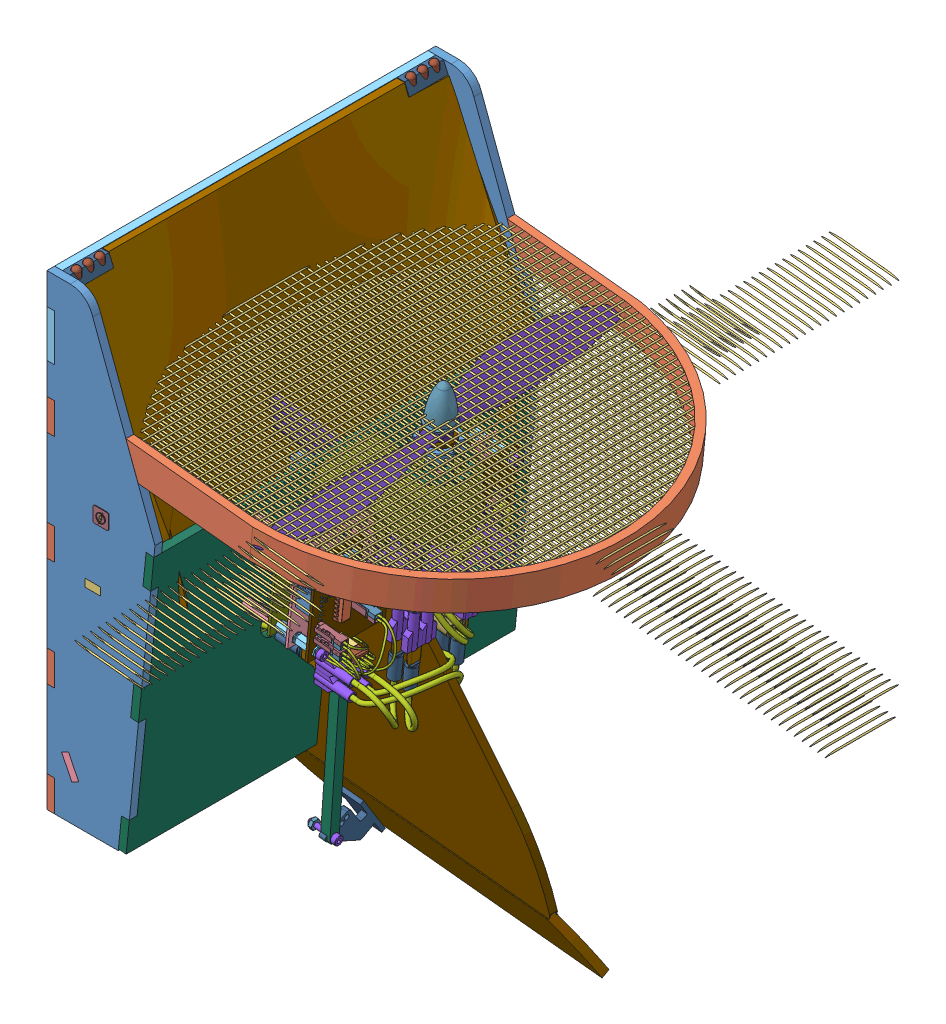
SolidWorks assembly AssTotaleSimu, configuration Défaut. Lengths in mm. (continued)
Components (placement in the parent): (continued)
- AssStructSimu-1: AssStructSimu [Défaut] at (-125.7658 -1.8483 624.6548) x (1 0 0) z (0 0 -1) size (323.53 326.04 251.6) (continued)
  - AssCarte-1: AssCarte [Défaut] at (-42.8534 32.2132 302.028) x (-0.101852 0.9948 0) z (0.9948 0.101852 0) size (91.19 130.57 98.45) (continued)
    - carte_onduleur_v4-1: carte_onduleur_v4 [Défaut] at (-25.7639 0.8332 112.9379) size (66.52 130.57 82.34) (continued)
      - C_DEC_COM1-1: C_DEC_COM1 [Défaut] at (-15 -36 0.803) x (0 -1 0) z (0 0 1) size (2.34 1.04 0.5) (continued)
        - Open CASCADE STEP translator 6.8 1.6.1-1: Open CASCADE STEP translator 6.8 1.6.1 [Défaut] at origin size (2.34 1.04 0.5)
          - Body_1-1: Body_1 [Défaut] at origin size (2.29 1.04 0.43)
          - Pin_1-1: Pin_1 [Défaut] at (0.3048 0 0) x (-1 0 0) z (0 0 1) size (0.51 1.02 0.5)
          - Pin_2-1: Pin_2 [Défaut] at origin size (0.51 1.02 0.5)
      - C_DEC_COMP2-1: C_DEC_COMP2 [Défaut] at (-13 -9.3 0.803) x (0 -1 0) z (0 0 1) size (2.34 1.04 0.5)
        - Open CASCADE STEP translator 6.8 1.6.1-1: Open CASCADE STEP translator 6.8 1.6.1 [Défaut] at origin size (2.34 1.04 0.5)
          - Body_1-1: Body_1 [Défaut] at origin size (2.29 1.04 0.43)
          - Pin_1-1: Pin_1 [Défaut] at (0.3048 0 0) x (-1 0 0) z (0 0 1) size (0.51 1.02 0.5)
          - Pin_2-1: Pin_2 [Défaut] at origin size (0.51 1.02 0.5)
      - C_DEC_COMP3-1: C_DEC_COMP3 [Défaut] at (-14.6 -22.9 0.803) x (0 -1 0) z (0 0 1) size (2.34 1.04 0.5)
        - Open CASCADE STEP translator 6.8 1.6.1-1: Open CASCADE STEP translator 6.8 1.6.1 [Défaut] at origin size (2.34 1.04 0.5)
          - Body_1-1: Body_1 [Défaut] at origin size (2.29 1.04 0.43)
          - Pin_1-1: Pin_1 [Défaut] at (0.3048 0 0) x (-1 0 0) z (0 0 1) size (0.51 1.02 0.5)
          - Pin_2-1: Pin_2 [Défaut] at origin size (0.51 1.02 0.5)
      - D_VBAT-1: D_VBAT [Défaut] at (-1.2 46.4 0.803) x (0 -1 0) z (0 0 1) size (2.34 1.04 0.5)
        - Open CASCADE STEP translator 6.8 1.6.1-1: Open CASCADE STEP translator 6.8 1.6.1 [Défaut] at origin size (2.34 1.04 0.5)
          - Body_1-1: Body_1 [Défaut] at origin size (2.29 1.04 0.43)
          - Pin_1-1: Pin_1 [Défaut] at (0.3048 0 0) x (-1 0 0) z (0 0 1) size (0.51 1.02 0.5)
          - Pin_2-1: Pin_2 [Défaut] at origin size (0.51 1.02 0.5)
      - D_3V-1: D_3V [Défaut] at (1.3 46.3 0.803) x (0 -1 0) z (0 0 1) size (2.34 1.04 0.5)
        - Open CASCADE STEP translator 6.8 1.6.1-1: Open CASCADE STEP translator 6.8 1.6.1 [Défaut] at origin size (2.34 1.04 0.5)
          - Body_1-1: Body_1 [Défaut] at origin size (2.29 1.04 0.43)
          - Pin_1-1: Pin_1 [Défaut] at (0.3048 0 0) x (-1 0 0) z (0 0 1) size (0.51 1.02 0.5)
          - Pin_2-1: Pin_2 [Défaut] at origin size (0.51 1.02 0.5)
      - D_5V-1: D_5V [Défaut] at (-3.7 46.4 0.803) x (0 -1 0) z (0 0 1) size (2.34 1.04 0.5)
        - Open CASCADE STEP translator 6.8 1.6.1-1: Open CASCADE STEP translator 6.8 1.6.1 [Défaut] at origin size (2.34 1.04 0.5)
          - Body_1-1: Body_1 [Défaut] at origin size (2.29 1.04 0.43)
          - Pin_1-1: Pin_1 [Défaut] at (0.3048 0 0) x (-1 0 0) z (0 0 1) size (0.51 1.02 0.5)
          - Pin_2-1: Pin_2 [Défaut] at origin size (0.51 1.02 0.5)
      - R1_1-1: R1_1 [Défaut] at (-20.2 -36.1 0.803) x (-1 0 0) z (0 0 1) size (2.34 1.04 0.5)
        - Open CASCADE STEP translator 6.8 1.12.1-1: Open CASCADE STEP translator 6.8 1.12.1 [Défaut] at origin size (2.34 1.04 0.5)
          - Body_1_3-1: Body_1_3 [Défaut] at origin size (2.29 1.04 0.43)
          - Pin_1_2-1: Pin_1_2 [Défaut] at (0.3048 0 0) x (-1 0 0) z (0 0 1) size (0.51 1.02 0.5)
          - Pin_2_2-1: Pin_2_2 [Défaut] at origin size (0.51 1.02 0.5)
      - R1_2-1: R1_2 [Défaut] at (-15.5 -34.6 0.803) x (-1 0 0) z (0 0 1) size (2.34 1.04 0.5)
        - Open CASCADE STEP translator 6.8 1.12.1-1: Open CASCADE STEP translator 6.8 1.12.1 [Défaut] at origin size (2.34 1.04 0.5)
          - Body_1_3-1: Body_1_3 [Défaut] at origin size (2.29 1.04 0.43)
          - Pin_1_2-1: Pin_1_2 [Défaut] at (0.3048 0 0) x (-1 0 0) z (0 0 1) size (0.51 1.02 0.5)
          - Pin_2_2-1: Pin_2_2 [Défaut] at origin size (0.51 1.02 0.5)
      - R1_3-1: R1_3 [Défaut] at (-20.3 -39.9 0.803) x (-1 0 0) z (0 0 1) size (2.34 1.04 0.5)
        - Open CASCADE STEP translator 6.8 1.12.1-1: Open CASCADE STEP translator 6.8 1.12.1 [Défaut] at origin size (2.34 1.04 0.5)
          - Body_1_3-1: Body_1_3 [Défaut] at origin size (2.29 1.04 0.43)
          - Pin_1_2-1: Pin_1_2 [Défaut] at (0.3048 0 0) x (-1 0 0) z (0 0 1) size (0.51 1.02 0.5)
          - Pin_2_2-1: Pin_2_2 [Défaut] at origin size (0.51 1.02 0.5)
      - R1_4-1: R1_4 [Défaut] at (-20.3 -38.1 0.803) x (-1 0 0) z (0 0 1) size (2.34 1.04 0.5)
        - Open CASCADE STEP translator 6.8 1.12.1-1: Open CASCADE STEP translator 6.8 1.12.1 [Défaut] at origin size (2.34 1.04 0.5)
          - Body_1_3-1: Body_1_3 [Défaut] at origin size (2.29 1.04 0.43)
          - Pin_1_2-1: Pin_1_2 [Défaut] at (0.3048 0 0) x (-1 0 0) z (0 0 1) size (0.51 1.02 0.5)
          - Pin_2_2-1: Pin_2_2 [Défaut] at origin size (0.51 1.02 0.5)
      - R1_5-1: R1_5 [Défaut] at (-17.1336 -39.7 0.803) size (2.34 1.04 0.5)
        - Open CASCADE STEP translator 6.8 1.12.1-1: Open CASCADE STEP translator 6.8 1.12.1 [Défaut] at origin size (2.34 1.04 0.5)
          - Body_1_3-1: Body_1_3 [Défaut] at origin size (2.29 1.04 0.43)
          - Pin_1_2-1: Pin_1_2 [Défaut] at (0.3048 0 0) x (-1 0 0) z (0 0 1) size (0.51 1.02 0.5)
          - Pin_2_2-1: Pin_2_2 [Défaut] at origin size (0.51 1.02 0.5)
      - R2_1-1: R2_1 [Défaut] at (-18.5 -9.5 0.803) x (-1 0 0) z (0 0 1) size (2.34 1.04 0.5)
        - Open CASCADE STEP translator 6.8 1.12.1-1: Open CASCADE STEP translator 6.8 1.12.1 [Défaut] at origin size (2.34 1.04 0.5)
          - Body_1_3-1: Body_1_3 [Défaut] at origin size (2.29 1.04 0.43)
          - Pin_1_2-1: Pin_1_2 [Défaut] at (0.3048 0 0) x (-1 0 0) z (0 0 1) size (0.51 1.02 0.5)
          - Pin_2_2-1: Pin_2_2 [Défaut] at origin size (0.51 1.02 0.5)
      - R2_2-1: R2_2 [Défaut] at (-13.1 -8 0.803) x (-1 0 0) z (0 0 1) size (2.34 1.04 0.5)
        - Open CASCADE STEP translator 6.8 1.12.1-1: Open CASCADE STEP translator 6.8 1.12.1 [Défaut] at origin size (2.34 1.04 0.5)
          - Body_1_3-1: Body_1_3 [Défaut] at origin size (2.29 1.04 0.43)
          - Pin_1_2-1: Pin_1_2 [Défaut] at (0.3048 0 0) x (-1 0 0) z (0 0 1) size (0.51 1.02 0.5)
          - Pin_2_2-1: Pin_2_2 [Défaut] at origin size (0.51 1.02 0.5)
      - R2_3-1: R2_3 [Défaut] at (-18.5 -11.2 0.803) x (-1 0 0) z (0 0 1) size (2.34 1.04 0.5)
        - Open CASCADE STEP translator 6.8 1.12.1-1: Open CASCADE STEP translator 6.8 1.12.1 [Défaut] at origin size (2.34 1.04 0.5)
          - Body_1_3-1: Body_1_3 [Défaut] at origin size (2.29 1.04 0.43)
          - Pin_1_2-1: Pin_1_2 [Défaut] at (0.3048 0 0) x (-1 0 0) z (0 0 1) size (0.51 1.02 0.5)
          - Pin_2_2-1: Pin_2_2 [Défaut] at origin size (0.51 1.02 0.5)
      - R2_4-1: R2_4 [Défaut] at (-18.5 -12.8 0.803) x (-1 0 0) z (0 0 1) size (2.34 1.04 0.5)
        - Open CASCADE STEP translator 6.8 1.12.1-1: Open CASCADE STEP translator 6.8 1.12.1 [Défaut] at origin size (2.34 1.04 0.5)
          - Body_1_3-1: Body_1_3 [Défaut] at origin size (2.29 1.04 0.43)
          - Pin_1_2-1: Pin_1_2 [Défaut] at (0.3048 0 0) x (-1 0 0) z (0 0 1) size (0.51 1.02 0.5)
          - Pin_2_2-1: Pin_2_2 [Défaut] at origin size (0.51 1.02 0.5)
      - R2_5-1: R2_5 [Défaut] at (-15.1336 -13 0.803) size (2.34 1.04 0.5)
        - Open CASCADE STEP translator 6.8 1.12.1-1: Open CASCADE STEP translator 6.8 1.12.1 [Défaut] at origin size (2.34 1.04 0.5)
          - Body_1_3-1: Body_1_3 [Défaut] at origin size (2.29 1.04 0.43)
          - Pin_1_2-1: Pin_1_2 [Défaut] at (0.3048 0 0) x (-1 0 0) z (0 0 1) size (0.51 1.02 0.5)
          - Pin_2_2-1: Pin_2_2 [Défaut] at origin size (0.51 1.02 0.5)
      - R3_1-1: R3_1 [Défaut] at (-19.9 -23.1 0.803) x (-1 0 0) z (0 0 1) size (2.34 1.04 0.5)
        - Open CASCADE STEP translator 6.8 1.12.1-1: Open CASCADE STEP translator 6.8 1.12.1 [Défaut] at origin size (2.34 1.04 0.5)
          - Body_1_3-1: Body_1_3 [Défaut] at origin size (2.29 1.04 0.43)
          - Pin_1_2-1: Pin_1_2 [Défaut] at (0.3048 0 0) x (-1 0 0) z (0 0 1) size (0.51 1.02 0.5)
          - Pin_2_2-1: Pin_2_2 [Défaut] at origin size (0.51 1.02 0.5)
      - R3_2-1: R3_2 [Défaut] at (-14.7 -21.6 0.803) x (-1 0 0) z (0 0 1) size (2.34 1.04 0.5)
        - Open CASCADE STEP translator 6.8 1.12.1-1: Open CASCADE STEP translator 6.8 1.12.1 [Défaut] at origin size (2.34 1.04 0.5)
          - Body_1_3-1: Body_1_3 [Défaut] at origin size (2.29 1.04 0.43)
          - Pin_1_2-1: Pin_1_2 [Défaut] at (0.3048 0 0) x (-1 0 0) z (0 0 1) size (0.51 1.02 0.5)
          - Pin_2_2-1: Pin_2_2 [Défaut] at origin size (0.51 1.02 0.5)
      - R3_3-1: R3_3 [Défaut] at (-19.9 -24.8 0.803) x (-1 0 0) z (0 0 1) size (2.34 1.04 0.5)
        - Open CASCADE STEP translator 6.8 1.12.1-1: Open CASCADE STEP translator 6.8 1.12.1 [Défaut] at origin size (2.34 1.04 0.5)
          - Body_1_3-1: Body_1_3 [Défaut] at origin size (2.29 1.04 0.43)
          - Pin_1_2-1: Pin_1_2 [Défaut] at (0.3048 0 0) x (-1 0 0) z (0 0 1) size (0.51 1.02 0.5)
          - Pin_2_2-1: Pin_2_2 [Défaut] at origin size (0.51 1.02 0.5)
      - R3_4-1: R3_4 [Défaut] at (-19.9 -26.4 0.803) x (-1 0 0) z (0 0 1) size (2.34 1.04 0.5)
        - Open CASCADE STEP translator 6.8 1.12.1-1: Open CASCADE STEP translator 6.8 1.12.1 [Défaut] at origin size (2.34 1.04 0.5)
          - Body_1_3-1: Body_1_3 [Défaut] at origin size (2.29 1.04 0.43)
          - Pin_1_2-1: Pin_1_2 [Défaut] at (0.3048 0 0) x (-1 0 0) z (0 0 1) size (0.51 1.02 0.5)
          - Pin_2_2-1: Pin_2_2 [Défaut] at origin size (0.51 1.02 0.5)
      - R3_5-1: R3_5 [Défaut] at (-16.7336 -26.5 0.803) size (2.34 1.04 0.5)
        - Open CASCADE STEP translator 6.8 1.12.1-1: Open CASCADE STEP translator 6.8 1.12.1 [Défaut] at origin size (2.34 1.04 0.5)
          - Body_1_3-1: Body_1_3 [Défaut] at origin size (2.29 1.04 0.43)
          - Pin_1_2-1: Pin_1_2 [Défaut] at (0.3048 0 0) x (-1 0 0) z (0 0 1) size (0.51 1.02 0.5)
          - Pin_2_2-1: Pin_2_2 [Défaut] at origin size (0.51 1.02 0.5)
      - R_LED_3V3-1: R_LED_3V3 [Défaut] at (1.3 47.9 0.803) x (0 1 0) z (0 0 1) size (2.34 1.04 0.5)
        - Open CASCADE STEP translator 6.8 1.12.1-1: Open CASCADE STEP translator 6.8 1.12.1 [Défaut] at origin size (2.34 1.04 0.5)
          - Body_1_3-1: Body_1_3 [Défaut] at origin size (2.29 1.04 0.43)
          - Pin_1_2-1: Pin_1_2 [Défaut] at (0.3048 0 0) x (-1 0 0) z (0 0 1) size (0.51 1.02 0.5)
          - Pin_2_2-1: Pin_2_2 [Défaut] at origin size (0.51 1.02 0.5)
      - R_LED_5V-1: R_LED_5V [Défaut] at (-3.7 47.7 0.803) x (0 1 0) z (0 0 1) size (2.34 1.04 0.5)
        - Open CASCADE STEP translator 6.8 1.12.1-1: Open CASCADE STEP translator 6.8 1.12.1 [Défaut] at origin size (2.34 1.04 0.5)
          - Body_1_3-1: Body_1_3 [Défaut] at origin size (2.29 1.04 0.43)
          - Pin_1_2-1: Pin_1_2 [Défaut] at (0.3048 0 0) x (-1 0 0) z (0 0 1) size (0.51 1.02 0.5)
          - Pin_2_2-1: Pin_2_2 [Défaut] at origin size (0.51 1.02 0.5)
      - R_LED_VBAT-1: R_LED_VBAT [Défaut] at (-1.2 47.9 0.803) x (0 1 0) z (0 0 1) size (2.34 1.04 0.5)
        - Open CASCADE STEP translator 6.8 1.12.1-1: Open CASCADE STEP translator 6.8 1.12.1 [Défaut] at origin size (2.34 1.04 0.5)
          - Body_1_3-1: Body_1_3 [Défaut] at origin size (2.29 1.04 0.43)
          - Pin_1_2-1: Pin_1_2 [Défaut] at (0.3048 0 0) x (-1 0 0) z (0 0 1) size (0.51 1.02 0.5)
          - Pin_2_2-1: Pin_2_2 [Défaut] at origin size (0.51 1.02 0.5)
      - CARTE_ALIM-1: CARTE_ALIM [Défaut] at (-6.4 -57.2 0.803) size (60 130 18.35)
        - Open CASCADE STEP translator 6.8 1.63.1-1: Open CASCADE STEP translator 6.8 1.63.1 [Défaut] at origin size (60 130 18.35)
          - Body_1_6-1: Body_1_6 [Défaut] at (7 56 -12) size (60 130 18.35)
            - 1_3-1: 1_3 [Défaut] at origin size (60 130 1.61)
            - 13_3-1: 13_3 [Défaut] at (0.4717 -40.93 0.803) x (0 1 0) z (0 0 1) size (5.65 4.9 1.7)
              - =_[0_1_1_4]_3-1: =_[0_1_1_4]_3 [Défaut] at origin size (5.65 4.9 1.7)
                - 2-1: 2 [Défaut] at origin size (3.75 4.9 1.53)
                - 3-1: 3 [Défaut] at origin size (0.95 0.51 1.06)
                - 4-1: 4 [Défaut] at origin size (0.95 0.51 1.06)
                - 5_2-1: 5_2 [Défaut] at origin size (0.95 0.51 1.06)
                - 6-1: 6 [Défaut] at origin size (0.95 0.51 1.06)
                - 7-1: 7 [Défaut] at (10.8 -5.08 0) x (-1 0 0) z (0 0 1) size (0.95 0.51 1.06)
                - 8_2-1: 8_2 [Défaut] at (10.8 -2.54 0) x (-1 0 0) z (0 0 1) size (0.95 0.51 1.06)
                - 9-1: 9 [Défaut] at (10.8 0 0) x (-1 0 0) z (0 0 1) size (0.95 0.51 1.06)
                - 10-1: 10 [Défaut] at (10.8 2.54 0) x (-1 0 0) z (0 0 1) size (0.95 0.51 1.06)
                - 11_2-1: 11_2 [Défaut] at (5.4 -1.27 0) x (-1 0 0) z (0 0 1) size (4.25 2.34 1.06)
            - 18-1: 18 [Défaut] at (-2.5283 -37.23 0.803) x (0 -1 0) z (0 0 1) size (2.34 1.04 0.5)
              - =_[0_1_1_16]-1: =_[0_1_1_16] [Défaut] at origin size (2.34 1.04 0.5)
                - 14_2-1: 14_2 [Défaut] at origin size (2.29 1.04 0.43)
                - 15_2-1: 15_2 [Défaut] at (0.3048 0 0) x (-1 0 0) z (0 0 1) size (0.51 1.02 0.5)
                - 16_2-1: 16_2 [Défaut] at origin size (0.51 1.02 0.5)
            - 21_2-1: 21_2 [Défaut] at (-2.2263 -24.628 -0.803) x (1 0 0) z (0 0 -1) size (8.01 8 14.24)
              - =_[0_1_1_21]-1: =_[0_1_1_21] [Défaut] at origin size (8.01 8 14.24)
                - 19-1: 19 [Défaut] at (1.8 0 0) x (1 0 0) z (0 -1 0) size (8.01 14.24 8)
            - 23_2-1: 23_2 [Défaut] at (1.2381 -31.53 0.803) size (2.34 1.04 0.5)
              - =_[0_1_1_16]-1: =_[0_1_1_16] [Défaut] at origin size (2.34 1.04 0.5)
                - 14_2-1: 14_2 [Défaut] at origin size (2.29 1.04 0.43)
                - 15_2-1: 15_2 [Défaut] at (0.3048 0 0) x (-1 0 0) z (0 0 1) size (0.51 1.02 0.5)
                - 16_2-1: 16_2 [Défaut] at origin size (0.51 1.02 0.5)
            - 28-1: 28 [Défaut] at (5 29.8636 0.803) x (0 -1 0) z (0 0 1) size (3.35 1.3 0.55)
              - =_[0_1_1_25]_2-1: =_[0_1_1_25]_2 [Défaut] at origin size (3.35 1.3 0.55)
                - 24-1: 24 [Défaut] at origin size (3.3 1.3 0.48)
                - 25_2-1: 25_2 [Défaut] at (0.5588 0 0) x (-1 0 0) z (0 0 1) size (0.76 1.27 0.55)
                - 26_2-1: 26_2 [Défaut] at origin size (0.76 1.27 0.55)
            - 30-1: 30 [Défaut] at (6.7 29.8636 0.803) x (0 -1 0) z (0 0 1) size (2.34 1.04 0.5)
              - =_[0_1_1_16]-1: =_[0_1_1_16] [Défaut] at origin size (2.34 1.04 0.5)
                - 14_2-1: 14_2 [Défaut] at origin size (2.29 1.04 0.43)
                - 15_2-1: 15_2 [Défaut] at (0.3048 0 0) x (-1 0 0) z (0 0 1) size (0.51 1.02 0.5)
                - 16_2-1: 16_2 [Défaut] at origin size (0.51 1.02 0.5)
            - 35_2-1: 35_2 [Défaut] at (-2.5 -46.37 0.803) x (0 1 0) z (0 0 1) size (3.4 2.06 0.79)
              - =_[0_1_1_31]-1: =_[0_1_1_31] [Défaut] at origin size (3.4 2.06 0.79)
                - 31_2-1: 31_2 [Défaut] at origin size (3.3 2.06 0.69)
                - 32_3-1: 32_3 [Défaut] at (0.5588 0 0) x (-1 0 0) z (0 0 1) size (0.81 2.03 0.79)
                - 33_3-1: 33_3 [Défaut] at origin size (0.81 2.03 0.79)
            - 37-1: 37 [Défaut] at (5 31.43 0.803) x (0 1 0) z (0 0 1) size (2.34 1.04 0.5)
              - =_[0_1_1_16]-1: =_[0_1_1_16] [Défaut] at origin size (2.34 1.04 0.5)
                - 14_2-1: 14_2 [Défaut] at origin size (2.29 1.04 0.43)
                - 15_2-1: 15_2 [Défaut] at (0.3048 0 0) x (-1 0 0) z (0 0 1) size (0.51 1.02 0.5)
                - 16_2-1: 16_2 [Défaut] at origin size (0.51 1.02 0.5)
            - 39-1: 39 [Défaut] at (-0.2 35.63 0.803) x (-1 0 0) z (0 0 1) size (2.34 1.04 0.5)
              - =_[0_1_1_16]-1: =_[0_1_1_16] [Défaut] at origin size (2.34 1.04 0.5)
                - 14_2-1: 14_2 [Défaut] at origin size (2.29 1.04 0.43)
                - 15_2-1: 15_2 [Défaut] at (0.3048 0 0) x (-1 0 0) z (0 0 1) size (0.51 1.02 0.5)
                - 16_2-1: 16_2 [Défaut] at origin size (0.51 1.02 0.5)
            - 41-1: 41 [Défaut] at (2.9 -45.5036 0.803) x (0 1 0) z (0 0 1) size (2.34 1.04 0.5)
              - =_[0_1_1_16]-1: =_[0_1_1_16] [Défaut] at origin size (2.34 1.04 0.5)
                - 14_2-1: 14_2 [Défaut] at origin size (2.29 1.04 0.43)
                - 15_2-1: 15_2 [Défaut] at (0.3048 0 0) x (-1 0 0) z (0 0 1) size (0.51 1.02 0.5)
                - 16_2-1: 16_2 [Défaut] at origin size (0.51 1.02 0.5)
            - 43-1: 43 [Défaut] at (17.1348 -42.6272 0.803) x (0 1 0) z (0 0 1) size (2.34 1.04 0.5)
              - =_[0_1_1_16]-1: =_[0_1_1_16] [Défaut] at origin size (2.34 1.04 0.5)
                - 14_2-1: 14_2 [Défaut] at origin size (2.29 1.04 0.43)
                - 15_2-1: 15_2 [Défaut] at (0.3048 0 0) x (-1 0 0) z (0 0 1) size (0.51 1.02 0.5)
                - 16_2-1: 16_2 [Défaut] at origin size (0.51 1.02 0.5)
            - 48_2-1: 48_2 [Défaut] at (-5.4717 -39.01 0.803) x (-1 0 0) z (0 0 1) size (4.19 3.4 1.75)
              - =_[0_1_1_40]-1: =_[0_1_1_40] [Défaut] at origin size (4.19 3.4 1.75)
                - 44_2-1: 44_2 [Défaut] at origin size (3.75 3.38 1.73)
                - 45_2-1: 45_2 [Défaut] at (0.438 0 0) x (-1 0 0) z (0 0 1) size (0.53 3.4 1.75)
                - 46-1: 46 [Défaut] at origin size (0.52 3.4 1.75)
            - 53-1: 53 [Défaut] at (0.9 35.63 0.803) size (2.34 1.04 0.5)
              - =_[0_1_1_45]-1: =_[0_1_1_45] [Défaut] at origin size (2.34 1.04 0.5)
                - 49_3-1: 49_3 [Défaut] at origin size (2.29 1.04 0.43)
                - 50-1: 50 [Défaut] at (0.3048 0 0) x (-1 0 0) z (0 0 1) size (0.51 1.02 0.5)
                - 51-1: 51 [Défaut] at origin size (0.51 1.02 0.5)
            - 55_2-1: 55_2 [Défaut] at (1.3 -45.5036 0.803) x (0 1 0) z (0 0 1) size (2.34 1.04 0.5)
              - =_[0_1_1_45]-1: =_[0_1_1_45] [Défaut] at origin size (2.34 1.04 0.5)
                - 49_3-1: 49_3 [Défaut] at origin size (2.29 1.04 0.43)
                - 50-1: 50 [Défaut] at (0.3048 0 0) x (-1 0 0) z (0 0 1) size (0.51 1.02 0.5)
                - 51-1: 51 [Défaut] at origin size (0.51 1.02 0.5)
            - 57_3-1: 57_3 [Défaut] at (17.2348 -43.9936 0.803) x (0 -1 0) z (0 0 1) size (2.34 1.04 0.5)
              - =_[0_1_1_45]-1: =_[0_1_1_45] [Défaut] at origin size (2.34 1.04 0.5)
                - 49_3-1: 49_3 [Défaut] at origin size (2.29 1.04 0.43)
                - 50-1: 50 [Défaut] at (0.3048 0 0) x (-1 0 0) z (0 0 1) size (0.51 1.02 0.5)
                - 51-1: 51 [Défaut] at origin size (0.51 1.02 0.5)
            - 65-1: 65 [Défaut] at (-4.8 30.93 0.803) x (-1 0 0) z (0 0 1) size (14.64 9.83 4.25)
              - =_[0_1_1_52]-1: =_[0_1_1_52] [Défaut] at origin size (14.64 9.83 4.25)
                - 63_2-1: 63_2 [Défaut] at (3 0 0) x (0 -1 0) z (0 0 1) size (9.83 14.64 4.25)
                  - =_[0_1_1_3]_5-1: =_[0_1_1_3]_5 [Défaut] at origin size (9.83 9.05 4.21)
                  - =_[0_1_1_4]_5-1: =_[0_1_1_4]_5 [Défaut] at origin size (9.48 7.76 1.21)
                  - =_[0_1_1_5]_5-1: =_[0_1_1_5]_5 [Défaut] at origin size (1.36 6.01 3.08)
                  - =_[0_1_1_6]_3-1: =_[0_1_1_6]_3 [Défaut] at origin size (1.36 6.01 3.08)
                  - =_[0_1_1_7]_3-1: =_[0_1_1_7]_3 [Défaut] at origin size (1.06 6.01 3.08)
            - 67-1: 67 [Défaut] at (13.5933 -37.5272 0.803) x (-1 0 0) z (0 0 1) size (2.34 1.04 0.5)
              - =_[0_1_1_16]-1: =_[0_1_1_16] [Défaut] at origin size (2.34 1.04 0.5)
                - 14_2-1: 14_2 [Défaut] at origin size (2.29 1.04 0.43)
                - 15_2-1: 15_2 [Défaut] at (0.3048 0 0) x (-1 0 0) z (0 0 1) size (0.51 1.02 0.5)
                - 16_2-1: 16_2 [Défaut] at origin size (0.51 1.02 0.5)
            - 70_2-1: 70_2 [Défaut] at (18.2733 -29.7272 0.803) x (0 1 0) z (0 0 1) size (6.06 4.95 1.88)
              - =_[0_1_1_61]-1: =_[0_1_1_61] [Défaut] at origin size (6.06 4.95 1.88)
                - 68-1: 68 [Défaut] x (1 0 0) z (0 -1 0) size (6.06 1.88 4.95)
            - 83-1: 83 [Défaut] at (-21.2 -38.07 0.803) x (-1 0 0) z (0 0 1) size (2.7 5.2 1.11)
              - =_[0_1_1_64]-1: =_[0_1_1_64] [Défaut] at origin size (2.7 5.2 1.11)
                - 84_2-1: 84_2 [Défaut] at (1.2 -4 0) x (0 1 0) z (0 0 1) size (5.2 2.7 1.11)
                  - =_[0_1_1_3]_6-1: =_[0_1_1_3]_6 [Défaut] at origin size (0.39 0.64 0.01)
                  - =_[0_1_1_4]_6-1: =_[0_1_1_4]_6 [Défaut] at origin size (0.6 1.9 0.2)
                  - =_[0_1_1_5]_6-1: =_[0_1_1_5]_6 [Défaut] at origin size (0.21 0.08 0.01)
                  - =_[0_1_1_6]_4-1: =_[0_1_1_6]_4 [Défaut] at origin size (0.6 1.9 0.2)
                  - =_[0_1_1_7]_4-1: =_[0_1_1_7]_4 [Défaut] at origin size (0.46 0.68 0.01)
                  - =_[0_1_1_8]_3-1: =_[0_1_1_8]_3 [Défaut] at origin size (0.38 0.66 0.01)
                  - =_[0_1_1_9]_2-1: =_[0_1_1_9]_2 [Défaut] at origin size (0.2 0.62 0.01)
                  - =_[0_1_1_10]_2-1: =_[0_1_1_10]_2 [Défaut] at origin size (4 2.7 1.1)
                  - =_[0_1_1_11]_2-1: =_[0_1_1_11]_2 [Défaut] at origin size (0.46 0.63 0.01)
                  - =_[0_1_1_12]_2-1: =_[0_1_1_12]_2 [Défaut] at origin size (0.56 0.68 0.01)
            - 86_2-1: 86_2 [Défaut] at (12.8933 -35.4272 0.803) x (0 1 0) z (0 0 1) size (2.7 5.2 1.11)
              - =_[0_1_1_77]-1: =_[0_1_1_77] [Défaut] at origin size (2.7 5.2 1.11)
                - 84_2-1: 84_2 [Défaut] at (1.2 -4 0) x (0 1 0) z (0 0 1) size (5.2 2.7 1.11)
                  - =_[0_1_1_3]_6-1: =_[0_1_1_3]_6 [Défaut] at origin size (0.39 0.64 0.01)
                  - =_[0_1_1_4]_6-1: =_[0_1_1_4]_6 [Défaut] at origin size (0.6 1.9 0.2)
                  - =_[0_1_1_5]_6-1: =_[0_1_1_5]_6 [Défaut] at origin size (0.21 0.08 0.01)
                  - =_[0_1_1_6]_4-1: =_[0_1_1_6]_4 [Défaut] at origin size (0.6 1.9 0.2)
                  - =_[0_1_1_7]_4-1: =_[0_1_1_7]_4 [Défaut] at origin size (0.46 0.68 0.01)
                  - =_[0_1_1_8]_3-1: =_[0_1_1_8]_3 [Défaut] at origin size (0.38 0.66 0.01)
                  - =_[0_1_1_9]_2-1: =_[0_1_1_9]_2 [Défaut] at origin size (0.2 0.62 0.01)
                  - =_[0_1_1_10]_2-1: =_[0_1_1_10]_2 [Défaut] at origin size (4 2.7 1.1)
                  - =_[0_1_1_11]_2-1: =_[0_1_1_11]_2 [Défaut] at origin size (0.46 0.63 0.01)
                  - =_[0_1_1_12]_2-1: =_[0_1_1_12]_2 [Défaut] at origin size (0.56 0.68 0.01)
            - 92_2-1: 92_2 [Défaut] at (20.9933 -39.3272 0.803) x (0 -1 0) z (0 0 1) size (2.79 1.98 0.64)
              - =_[0_1_1_79]-1: =_[0_1_1_79] [Défaut] at origin size (2.79 1.98 0.64)
                - 87-1: 87 [Défaut] at origin size (2.79 1.02 0.58)
                - 88-1: 88 [Défaut] x (0 -1 0) z (0 0 1) size (0.42 0.38 0.38)
                - 89-1: 89 [Défaut] at (-2.8448 -0.9652 0) x (0 1 0) z (0 0 1) size (0.55 0.38 0.38)
                - 90-1: 90 [Défaut] at (-0.9652 -2.8448 0) x (0 1 0) z (0 0 1) size (0.55 0.38 0.38)
            - 98-1: 98 [Défaut] at (-17.7 -48.47 0.803) x (0 -1 0) z (0 0 1) size (2.54 1.98 0.64)
              - =_[0_1_1_85]-1: =_[0_1_1_85] [Défaut] at origin size (2.54 1.98 0.64)
                - 93-1: 93 [Défaut] at origin size (2.54 1.14 0.58)
                - 94-1: 94 [Défaut] x (0 -1 0) z (0 0 1) size (0.43 0.51 0.38)
                - 95-1: 95 [Défaut] at (1.8796 1.8796 0) x (0 -1 0) z (0 0 1) size (0.43 0.51 0.38)
                - 96-1: 96 [Défaut] at (-0.9652 -2.8448 0) x (0 1 0) z (0 0 1) size (0.41 0.51 0.38)
            - 100-1: 100 [Défaut] at (24.3933 -43.2272 0.803) size (2.79 1.98 0.64)
              - =_[0_1_1_79]-1: =_[0_1_1_79] [Défaut] at origin size (2.79 1.98 0.64)
                - 87-1: 87 [Défaut] at origin size (2.79 1.02 0.58)
                - 88-1: 88 [Défaut] x (0 -1 0) z (0 0 1) size (0.42 0.38 0.38)
                - 89-1: 89 [Défaut] at (-2.8448 -0.9652 0) x (0 1 0) z (0 0 1) size (0.55 0.38 0.38)
                - 90-1: 90 [Défaut] at (-0.9652 -2.8448 0) x (0 1 0) z (0 0 1) size (0.55 0.38 0.38)
            - 102-1: 102 [Défaut] at (21.4933 -44.4272 0.803) x (0 -1 0) z (0 0 1) size (2.79 1.98 0.64)
              - =_[0_1_1_79]-1: =_[0_1_1_79] [Défaut] at origin size (2.79 1.98 0.64)
                - 87-1: 87 [Défaut] at origin size (2.79 1.02 0.58)
                - 88-1: 88 [Défaut] x (0 -1 0) z (0 0 1) size (0.42 0.38 0.38)
                - 89-1: 89 [Défaut] at (-2.8448 -0.9652 0) x (0 1 0) z (0 0 1) size (0.55 0.38 0.38)
                - 90-1: 90 [Défaut] at (-0.9652 -2.8448 0) x (0 1 0) z (0 0 1) size (0.55 0.38 0.38)
            - 107-1: 107 [Défaut] at (23.1933 -29.1272 -0.803) x (0 1 0) z (0 0 -1) size (9.6 14.35 5)
              - =_[0_1_1_93]-1: =_[0_1_1_93] [Défaut] at origin size (9.6 14.35 5)
                - 105-1: 105 [Défaut] at (0.5 -1 2) x (-1 0 0) z (0 0 1) size (9.6 14.35 5)
                  - =_[0_1_1_3]_7-1: =_[0_1_1_3]_7 [Défaut] at origin size (9.6 12.75 5)
                  - =_[0_1_1_4]_7-1: =_[0_1_1_4]_7 [Défaut] at origin size (2.2 1.6 2.2)
            - 109-1: 109 [Défaut] at (25.4933 -41.1272 0.803) x (-1 0 0) z (0 0 1) size (2.34 1.04 0.5)
              - =_[0_1_1_45]-1: =_[0_1_1_45] [Défaut] at origin size (2.34 1.04 0.5)
                - 49_3-1: 49_3 [Défaut] at origin size (2.29 1.04 0.43)
                - 50-1: 50 [Défaut] at (0.3048 0 0) x (-1 0 0) z (0 0 1) size (0.51 1.02 0.5)
                - 51-1: 51 [Défaut] at origin size (0.51 1.02 0.5)
            - 111-1: 111 [Défaut] at (22.0269 -41.8272 0.803) x (-1 0 0) z (0 0 1) size (2.34 1.04 0.5)
              - =_[0_1_1_45]-1: =_[0_1_1_45] [Défaut] at origin size (2.34 1.04 0.5)
                - 49_3-1: 49_3 [Défaut] at origin size (2.29 1.04 0.43)
                - 50-1: 50 [Défaut] at (0.3048 0 0) x (-1 0 0) z (0 0 1) size (0.51 1.02 0.5)
                - 51-1: 51 [Défaut] at origin size (0.51 1.02 0.5)
            - 113-1: 113 [Défaut] at (-24.8 -36.7036 0.803) x (0 1 0) z (0 0 1) size (2.34 1.04 0.5)
              - =_[0_1_1_45]-1: =_[0_1_1_45] [Défaut] at origin size (2.34 1.04 0.5)
                - 49_3-1: 49_3 [Défaut] at origin size (2.29 1.04 0.43)
                - 50-1: 50 [Défaut] at (0.3048 0 0) x (-1 0 0) z (0 0 1) size (0.51 1.02 0.5)
                - 51-1: 51 [Défaut] at origin size (0.51 1.02 0.5)
            - 115-1: 115 [Défaut] at (-24.8 -40.3036 0.803) x (0 1 0) z (0 0 1) size (2.34 1.04 0.5)
              - =_[0_1_1_45]-1: =_[0_1_1_45] [Défaut] at origin size (2.34 1.04 0.5)
                - 49_3-1: 49_3 [Défaut] at origin size (2.29 1.04 0.43)
                - 50-1: 50 [Défaut] at (0.3048 0 0) x (-1 0 0) z (0 0 1) size (0.51 1.02 0.5)
                - 51-1: 51 [Défaut] at origin size (0.51 1.02 0.5)
            - 117-1: 117 [Défaut] at (-16 -48.27 0.803) x (0 -1 0) z (0 0 1) size (2.34 1.04 0.5)
              - =_[0_1_1_45]-1: =_[0_1_1_45] [Défaut] at origin size (2.34 1.04 0.5)
                - 49_3-1: 49_3 [Défaut] at origin size (2.29 1.04 0.43)
                - 50-1: 50 [Défaut] at (0.3048 0 0) x (-1 0 0) z (0 0 1) size (0.51 1.02 0.5)
                - 51-1: 51 [Défaut] at origin size (0.51 1.02 0.5)
            - 119-1: 119 [Défaut] at (-22.5189 -47.87 0.803) x (-1 0 0) z (0 0 1) size (2.34 1.04 0.5)
              - =_[0_1_1_45]-1: =_[0_1_1_45] [Défaut] at origin size (2.34 1.04 0.5)
                - 49_3-1: 49_3 [Défaut] at origin size (2.29 1.04 0.43)
                - 50-1: 50 [Défaut] at (0.3048 0 0) x (-1 0 0) z (0 0 1) size (0.51 1.02 0.5)
                - 51-1: 51 [Défaut] at origin size (0.51 1.02 0.5)
            - 121-1: 121 [Défaut] at (22.3933 -38.9272 0.803) size (2.34 1.04 0.5)
              - =_[0_1_1_45]-1: =_[0_1_1_45] [Défaut] at origin size (2.34 1.04 0.5)
                - 49_3-1: 49_3 [Défaut] at origin size (2.29 1.04 0.43)
                - 50-1: 50 [Défaut] at (0.3048 0 0) x (-1 0 0) z (0 0 1) size (0.51 1.02 0.5)
                - 51-1: 51 [Défaut] at origin size (0.51 1.02 0.5)
            - 123-1: 123 [Défaut] at (22.0933 -36.4272 0.803) x (-1 0 0) z (0 0 1) size (2.34 1.04 0.5)
              - =_[0_1_1_45]-1: =_[0_1_1_45] [Défaut] at origin size (2.34 1.04 0.5)
                - 49_3-1: 49_3 [Défaut] at origin size (2.29 1.04 0.43)
                - 50-1: 50 [Défaut] at (0.3048 0 0) x (-1 0 0) z (0 0 1) size (0.51 1.02 0.5)
                - 51-1: 51 [Défaut] at origin size (0.51 1.02 0.5)
            - 125-1: 125 [Défaut] at (22.3933 -32.0272 0.803) x (0 -1 0) z (0 0 1) size (2.34 1.04 0.5)
              - =_[0_1_1_45]-1: =_[0_1_1_45] [Défaut] at origin size (2.34 1.04 0.5)
                - 49_3-1: 49_3 [Défaut] at origin size (2.29 1.04 0.43)
                - 50-1: 50 [Défaut] at (0.3048 0 0) x (-1 0 0) z (0 0 1) size (0.51 1.02 0.5)
                - 51-1: 51 [Défaut] at origin size (0.51 1.02 0.5)
            - 127-1: 127 [Défaut] at (17.9597 -23.1272 0.803) size (2.34 1.04 0.5)
              - =_[0_1_1_16]-1: =_[0_1_1_16] [Défaut] at origin size (2.34 1.04 0.5)
                - 14_2-1: 14_2 [Défaut] at origin size (2.29 1.04 0.43)
                - 15_2-1: 15_2 [Défaut] at (0.3048 0 0) x (-1 0 0) z (0 0 1) size (0.51 1.02 0.5)
                - 16_2-1: 16_2 [Défaut] at origin size (0.51 1.02 0.5)
            - 129-1: 129 [Défaut] at (20.0269 -24.9272 0.803) x (-1 0 0) z (0 0 1) size (2.34 1.04 0.5)
              - =_[0_1_1_16]-1: =_[0_1_1_16] [Défaut] at origin size (2.34 1.04 0.5)
                - 14_2-1: 14_2 [Défaut] at origin size (2.29 1.04 0.43)
                - 15_2-1: 15_2 [Défaut] at (0.3048 0 0) x (-1 0 0) z (0 0 1) size (0.51 1.02 0.5)
                - 16_2-1: 16_2 [Défaut] at origin size (0.51 1.02 0.5)
            - 131-1: 131 [Défaut] at (16.9933 -37.5272 0.803) x (-1 0 0) z (0 0 1) size (2.34 1.04 0.5)
              - =_[0_1_1_45]-1: =_[0_1_1_45] [Défaut] at origin size (2.34 1.04 0.5)
                - 49_3-1: 49_3 [Défaut] at origin size (2.29 1.04 0.43)
                - 50-1: 50 [Défaut] at (0.3048 0 0) x (-1 0 0) z (0 0 1) size (0.51 1.02 0.5)
                - 51-1: 51 [Défaut] at origin size (0.51 1.02 0.5)
            - 136-1: 136 [Défaut] at (3.2957 -29.23 0.803) x (-1 0 0) z (0 0 1) size (4.78 2.79 2.03)
              - =_[0_1_1_110]_2-1: =_[0_1_1_110]_2 [Défaut] at origin size (4.78 2.79 2.03)
                - 132-1: 132 [Défaut] at origin size (4.32 2.79 1.78)
                - 133-1: 133 [Défaut] at (0.4572 0 0) x (-1 0 0) z (0 0 1) size (1.02 1.27 1.32)
                - 134-1: 134 [Défaut] at origin size (1.02 1.27 1.32)
            - 141-1: 141 [Défaut] at (0.2436 -33.3673 0.803) size (3.35 1.3 0.55)
              - =_[0_1_1_115]_2-1: =_[0_1_1_115]_2 [Défaut] at origin size (3.35 1.3 0.55)
                - 137-1: 137 [Défaut] at origin size (3.3 1.3 0.48)
                - 138-1: 138 [Défaut] at (0.5588 0 0) x (-1 0 0) z (0 0 1) size (0.76 1.27 0.55)
                - 139-1: 139 [Défaut] at origin size (0.76 1.27 0.55)
            - 143_2-1: 143_2 [Défaut] at (-0.3 -45.47 0.803) x (0 1 0) z (0 0 1) size (2.34 1.04 0.5)
              - =_[0_1_1_16]-1: =_[0_1_1_16] [Défaut] at origin size (2.34 1.04 0.5)
                - 14_2-1: 14_2 [Défaut] at origin size (2.29 1.04 0.43)
                - 15_2-1: 15_2 [Défaut] at (0.3048 0 0) x (-1 0 0) z (0 0 1) size (0.51 1.02 0.5)
                - 16_2-1: 16_2 [Défaut] at origin size (0.51 1.02 0.5)
            - 145-1: 145 [Défaut] at (6.6 31.13 0.803) x (0 1 0) z (0 0 1) size (3.35 1.3 0.55)
              - =_[0_1_1_25]_2-1: =_[0_1_1_25]_2 [Défaut] at origin size (3.35 1.3 0.55)
                - 24-1: 24 [Défaut] at origin size (3.3 1.3 0.48)
                - 25_2-1: 25_2 [Défaut] at (0.5588 0 0) x (-1 0 0) z (0 0 1) size (0.76 1.27 0.55)
                - 26_2-1: 26_2 [Défaut] at origin size (0.76 1.27 0.55)
            - 148-1: 148 [Défaut] at (-7.5 -56.57 0.803) size (15.24 2.54 7.37)
              - =_[0_1_1_122]_2-1: =_[0_1_1_122]_2 [Défaut] at origin size (15.24 2.54 7.37)
                - 146-1: 146 [Défaut] at (6.3 0 1) x (1 0 0) z (0 -1 0) size (15.24 7.37 2.54)
            - 150-1: 150 [Défaut] at (-26.3 -45.9 0.803) x (0 1 0) z (0 0 1) size (2.34 1.04 0.5)
              - =_[0_1_1_45]-1: =_[0_1_1_45] [Défaut] at origin size (2.34 1.04 0.5)
                - 49_3-1: 49_3 [Défaut] at origin size (2.29 1.04 0.43)
                - 50-1: 50 [Défaut] at (0.3048 0 0) x (-1 0 0) z (0 0 1) size (0.51 1.02 0.5)
                - 51-1: 51 [Défaut] at origin size (0.51 1.02 0.5)
    - AssEntretoise-1: AssEntretoise [Défaut] at (-50.7639 -62.5535 129.2811) x (0 0 -1) z (1 0 0) size (58.24 7.29 7.81)
      - socket head cap screw 4762_din-1: socket head cap screw 4762_din [EN ISO 4762 M3 x 5 - 5N] at (-2.4967 0.5867 0) size (8 5.5 5.5)
      - hexagonal_spacer_MF_M3_H20_HEX5.5_FTD6_MTL6-1: hexagonal_spacer_MF_M3_H20_HEX5.5_FTD6_MTL6 [Défaut] at (48.3433 0.5867 0) x (0 0 1) z (-1 0 0) size (6.36 5.51 26)
      - hex nut style 1 gradeab_din-1: hex nut style 1 gradeab_din [Hexagon Nut ISO 4032 - M3 - W - N] at (53.3433 0.5867 0) x (0 0.943962 0.330053) z (-1 0 0) size (5.5 6.35 2.4)
      - hexagonal_spacer_MF_M3_H12_HEX5.5_FTD6_MTL6-2: hexagonal_spacer_MF_M3_H12_HEX5.5_FTD6_MTL6 [Défaut] at (27.0633 0.5867 0) x (0 0.248308 0.968681) z (-1 0 0) size (6.36 5.51 18)
      - hexagonal_spacer_MF_M3_H12_HEX5.5_FTD6_MTL6-3: hexagonal_spacer_MF_M3_H12_HEX5.5_FTD6_MTL6 [Défaut] at (13.7833 0.5867 0) x (0 0 1) z (-1 0 0) size (6.36 5.51 18)
    - AssEntretoise-2: AssEntretoise [Défaut] at (0.4521 -62.0374 129.2811) x (0 0 -1) z (0.694658 0.71934 0) size (58.24 7.29 7.81)
      - socket head cap screw 4762_din-1: socket head cap screw 4762_din [EN ISO 4762 M3 x 5 - 5N] at (-2.4967 0.5867 0) size (8 5.5 5.5)
      - hexagonal_spacer_MF_M3_H20_HEX5.5_FTD6_MTL6-1: hexagonal_spacer_MF_M3_H20_HEX5.5_FTD6_MTL6 [Défaut] at (48.3433 0.5867 0) x (0 0 1) z (-1 0 0) size (6.36 5.51 26)
      - hex nut style 1 gradeab_din-1: hex nut style 1 gradeab_din [Hexagon Nut ISO 4032 - M3 - W - N] at (53.3433 0.5867 0) x (0 0.943962 0.330053) z (-1 0 0) size (5.5 6.35 2.4)
      - hexagonal_spacer_MF_M3_H12_HEX5.5_FTD6_MTL6-2: hexagonal_spacer_MF_M3_H12_HEX5.5_FTD6_MTL6 [Défaut] at (27.0633 0.5867 0) x (0 0.248308 0.968681) z (-1 0 0) size (6.36 5.51 18)
      - hexagonal_spacer_MF_M3_H12_HEX5.5_FTD6_MTL6-3: hexagonal_spacer_MF_M3_H12_HEX5.5_FTD6_MTL6 [Défaut] at (13.7833 0.5867 0) x (0 0 1) z (-1 0 0) size (6.36 5.51 18)
    - AssEntretoise-3: AssEntretoise [Défaut] at (-51.9799 58.1038 129.2811) x (0 0 -1) z (-0.694658 -0.71934 0) size (58.24 7.29 7.81)
      - socket head cap screw 4762_din-1: socket head cap screw 4762_din [EN ISO 4762 M3 x 5 - 5N] at (-2.4967 0.5867 0) size (8 5.5 5.5)
      - hexagonal_spacer_MF_M3_H20_HEX5.5_FTD6_MTL6-1: hexagonal_spacer_MF_M3_H20_HEX5.5_FTD6_MTL6 [Défaut] at (48.3433 0.5867 0) x (0 0 1) z (-1 0 0) size (6.36 5.51 26)
      - hex nut style 1 gradeab_din-1: hex nut style 1 gradeab_din [Hexagon Nut ISO 4032 - M3 - W - N] at (53.3433 0.5867 0) x (0 0.943962 0.330053) z (-1 0 0) size (5.5 6.35 2.4)
      - hexagonal_spacer_MF_M3_H12_HEX5.5_FTD6_MTL6-2: hexagonal_spacer_MF_M3_H12_HEX5.5_FTD6_MTL6 [Défaut] at (27.0633 0.5867 0) x (0 0.248308 0.968681) z (-1 0 0) size (6.36 5.51 18)
      - hexagonal_spacer_MF_M3_H12_HEX5.5_FTD6_MTL6-3: hexagonal_spacer_MF_M3_H12_HEX5.5_FTD6_MTL6 [Défaut] at (13.7833 0.5867 0) x (0 0 1) z (-1 0 0) size (6.36 5.51 18)
    - AssEntretoise-4: AssEntretoise [Défaut] at (0.2897 58.1744 129.2811) x (0 0 -1) z (-0.999848 0.017452 0) size (58.24 7.29 7.81)
      - socket head cap screw 4762_din-1: socket head cap screw 4762_din [EN ISO 4762 M3 x 5 - 5N] at (-2.4967 0.5867 0) size (8 5.5 5.5)
      - hexagonal_spacer_MF_M3_H20_HEX5.5_FTD6_MTL6-1: hexagonal_spacer_MF_M3_H20_HEX5.5_FTD6_MTL6 [Défaut] at (48.3433 0.5867 0) x (0 0 1) z (-1 0 0) size (6.36 5.51 26)
      - hex nut style 1 gradeab_din-1: hex nut style 1 gradeab_din [Hexagon Nut ISO 4032 - M3 - W - N] at (53.3433 0.5867 0) x (0 0.943962 0.330053) z (-1 0 0) size (5.5 6.35 2.4)
      - hexagonal_spacer_MF_M3_H12_HEX5.5_FTD6_MTL6-2: hexagonal_spacer_MF_M3_H12_HEX5.5_FTD6_MTL6 [Défaut] at (27.0633 0.5867 0) x (0 0.248308 0.968681) z (-1 0 0) size (6.36 5.51 18)
      - hexagonal_spacer_MF_M3_H12_HEX5.5_FTD6_MTL6-3: hexagonal_spacer_MF_M3_H12_HEX5.5_FTD6_MTL6 [Défaut] at (13.7833 0.5867 0) x (0 0 1) z (-1 0 0) size (6.36 5.51 18)
    - AssMpu-1: AssMpu [Défaut] at (-44.7921 29.4106 121.7839) size (8 8 22.28)
      - hex nut style 1 gradeab_din-1: hex nut style 1 gradeab_din [Hexagon Nut ISO 4032 - M3 - W - N] at (0.2783 0.3227 1.2) size (5.5 6.35 2.4)
      - plain washer 6903 type ab_din-1: plain washer 6903 type ab_din [DIN 6903-A3] at (0.2783 0.3227 1.2) x (0 0 1) z (-1 0 0) size (1 8 8)
      - socket head cap screw 4762_din-1: socket head cap screw 4762_din [EN ISO 4762 M3 x 5 - 5N] at (0.2783 0.3227 19.76) x (0 0 -1) z (-0.852155 0.523289 0) size (8 5.5 5.5)
      - hexagonal_spacer_MF_M3_H12_HEX5.5_FTD6_MTL6-1: hexagonal_spacer_MF_M3_H12_HEX5.5_FTD6_MTL6 [Défaut] at (0.2783 0.3227 3.48) size (6.36 5.51 18)
    - AssMpu-2: AssMpu [Défaut] at (-24.7921 29.4106 121.7839) size (8 8 22.28)
      - hex nut style 1 gradeab_din-1: hex nut style 1 gradeab_din [Hexagon Nut ISO 4032 - M3 - W - N] at (0.2783 0.3227 1.2) size (5.5 6.35 2.4)
      - plain washer 6903 type ab_din-1: plain washer 6903 type ab_din [DIN 6903-A3] at (0.2783 0.3227 1.2) x (0 0 1) z (-1 0 0) size (1 8 8)
      - socket head cap screw 4762_din-1: socket head cap screw 4762_din [EN ISO 4762 M3 x 5 - 5N] at (0.2783 0.3227 19.76) x (0 0 -1) z (-0.852155 0.523289 0) size (8 5.5 5.5)
      - hexagonal_spacer_MF_M3_H12_HEX5.5_FTD6_MTL6-1: hexagonal_spacer_MF_M3_H12_HEX5.5_FTD6_MTL6 [Défaut] at (0.2783 0.3227 3.48) size (6.36 5.51 18)
    - AssCosse-1: AssCosse [Défaut] at (-36.6204 16.2367 163.5671) x (0 1 0) z (-0.344896 0 0.938641) size (9.83 18.66 11.64)
      - socket head cap screw 4762_din-1: socket head cap screw 4762_din [EN ISO 4762 M3 x 6 - 6N] at (-5.1064 0.3659 0) size (9 5.5 5.5)
      - plain washer 6903 type ab_din-1: plain washer 6903 type ab_din [DIN 6903-A3] at (-2.1064 0.3659 0) size (1 8 8)
      - hex nut style 1 gradeab_din-2: hex nut style 1 gradeab_din [Hexagon Nut ISO 4032 - M3 - W - N] at (1.281 0.3659 0) x (0 0.924225 0.381849) z (-1 0 0) size (5.5 6.35 2.4)
      - 31880-1: 31880 [Default] at (0.4936 0.3659 0) x (0 0.344896 -0.938641) z (0 -0.938641 -0.344896) size (5.54 5 17.37)
    - AssCosse-2: AssCosse [Défaut] at (-36.6204 1.2367 163.5671) x (0 1 0) z (-0.344896 0 0.938641) size (9.83 18.66 11.64)
      - socket head cap screw 4762_din-1: socket head cap screw 4762_din [EN ISO 4762 M3 x 6 - 6N] at (-5.1064 0.3659 0) size (9 5.5 5.5)
      - plain washer 6903 type ab_din-1: plain washer 6903 type ab_din [DIN 6903-A3] at (-2.1064 0.3659 0) size (1 8 8)
      - hex nut style 1 gradeab_din-2: hex nut style 1 gradeab_din [Hexagon Nut ISO 4032 - M3 - W - N] at (1.281 0.3659 0) x (0 0.924225 0.381849) z (-1 0 0) size (5.5 6.35 2.4)
      - 31880-1: 31880 [Default] at (0.4936 0.3659 0) x (0 0.344896 -0.938641) z (0 -0.938641 -0.344896) size (5.54 5 17.37)
    - AssCosse-3: AssCosse [Défaut] at (-36.6204 -13.7633 163.5671) x (0 1 0) z (-0.344896 0 0.938641) size (9.83 18.66 11.64)
      - socket head cap screw 4762_din-1: socket head cap screw 4762_din [EN ISO 4762 M3 x 6 - 6N] at (-5.1064 0.3659 0) size (9 5.5 5.5)
